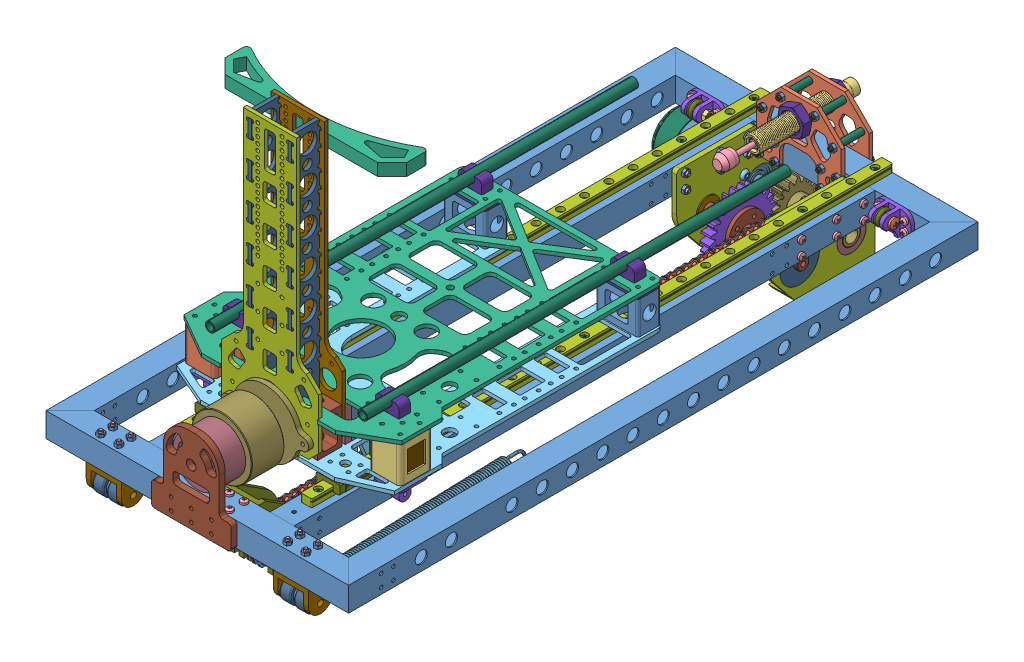
SolidWorks assembly 寒冰射手-wlⅡ-2AT-sc, configuration 默认. Lengths in mm.
Overall size (250 317.6 547).
340 component instances, 60 part files, 291 mates.
Components (placement in the parent):
- 发射架-wlⅡ-2AT-sc-1: 发射架-wlⅡ-2AT-sc [默认<按加工>] at (-51.2492 42.8186 0) size (250 20 520)
- 缓冲器固定板-wlⅡ-2AT-sc-1: 缓冲器固定板-wlⅡ-2AT-sc [默认] at (-86.2492 32.8186 -263) x (1 0 0) z (0 -1 0) size (70 3 58)
- 缓冲器固定板-wlⅡ-2AT-sc-3: 缓冲器固定板-wlⅡ-2AT-sc [默认] at (-86.2492 32.8186 -240) x (1 0 0) z (0 -1 0) size (70 3 58)
- 阻尼器-wlⅡ-2AT-sc-1: 阻尼器-wlⅡ-2AT-sc [默认] at (5.2053 79.9344 -231.7218) x (0.997955 0.063917 0) z (0.063917 -0.997955 0) size (16.63 112.5 16.63)
  - 阻尼器缸体-wlⅡ-2AT-sc-1: 阻尼器缸体-wlⅡ-2AT-sc [默认] at (-56.5702 -50.2782 0) size (16.17 84.55 14.32)
  - 阻尼器杆-wlⅡ-2AT-sc-1: 阻尼器杆-wlⅡ-2AT-sc [默认] at (-56.5702 14.7218 0) x (0.905287 0 0.424801) z (-0.424801 0 0.905287) size (12.5 47.5 12.5)
  - GB／T70．1-2000内六角圆柱头螺钉M4×20-wlⅡ-2AT-sc-1: GB／T70．1-2000内六角圆柱头螺钉M4×20-wlⅡ-2AT-sc [默认] at (-56.5702 -49.2782 0) x (0 1 0) z (0.698141 0 0.715961) size (24 7 7)
  - circlips for holes--type a gb-1: circlips for holes--type a gb [GB_CONNECTING_PIECE_RING_RRH 10] at (-56.5702 31.0218 0) x (1 0 0) z (0 1 0) size (10.8 10.39 0.8)
- 发射导轨-wlⅡ-2AT-sc-1: 发射导轨-wlⅡ-2AT-sc [默认] at (-1.2492 56.482 -260) size (9 6.5 480)
- 发射导轨-wlⅡ-2AT-sc-2: 发射导轨-wlⅡ-2AT-sc [默认] at (-101.2492 56.482 -260) size (9 6.5 480)
- 拉线座子-wlⅡ-2AT-sc-1: 拉线座子-wlⅡ-2AT-sc [默认] at (26.0008 25.8186 -231.5) x (-1 0 0) z (0 0 -1) size (30.5 20 17)
- 拉线座子-wlⅡ-2AT-sc-2: 拉线座子-wlⅡ-2AT-sc [默认] at (-128.4992 25.8186 -231.5) x (-1 0 0) z (0 0 -1) size (30.5 20 17)
- 拉簧座子-wlⅡ-2AT-sc-1: 拉簧座子-wlⅡ-2AT-sc [默认] at (26.0008 32.8186 250) x (0 0 -1) z (0 -1 0) size (20 29 22)
- 拉簧座子-wlⅡ-2AT-sc-2: 拉簧座子-wlⅡ-2AT-sc [默认] at (-128.4992 32.8186 250) x (0 0 -1) z (0 -1 0) size (20 29 22)
- 弹簧限位件-wlⅡ-2AT-sc-1: 弹簧限位件-wlⅡ-2AT-sc [Default] at (-129.9992 18.3186 250) x (0 0.381849 -0.924225) z (0 0.924225 0.381849) size (18 9 18)
- 弹簧限位件-wlⅡ-2AT-sc-2: 弹簧限位件-wlⅡ-2AT-sc [Default] at (-117.9992 18.3186 250) x (0 0.381849 -0.924225) z (0 0.924225 0.381849) size (18 9 18)
- 弹簧限位件-wlⅡ-2AT-sc-3: 弹簧限位件-wlⅡ-2AT-sc [Default] at (36.5008 18.3186 250) x (0 0.381849 -0.924225) z (0 0.924225 0.381849) size (18 9 18)
- 弹簧限位件-wlⅡ-2AT-sc-4: 弹簧限位件-wlⅡ-2AT-sc [Default] at (24.5008 18.3186 250) x (0 0.381849 -0.924225) z (0 0.924225 0.381849) size (18 9 18)
- 电磁吸盘固定板-wlⅡ-2AT-sc-1: 电磁吸盘固定板-wlⅡ-2AT-sc [默认] at (-51.2492 67.8186 265) x (1 0 0) z (0 1 0) size (66 5 70)
- 电磁铁开关80kg-wlⅡ-2AT-sc-1: 电磁铁开关80kg-wlⅡ-2AT-sc [默认] at (-51.2492 78.8186 213) x (-0.910179 -0.414215 0) z (-0.414215 0.910179 0) size (50 27 50)
- 行程调节块-wlⅡ-2AT-sc-1: 行程调节块-wlⅡ-2AT-sc [默认] at (-51.2492 78.8186 240) x (1 0 0) z (0 -1 0) size (40 20 40)
- 拉射拉簧-wlⅡ-2AT-sc-1: 拉射拉簧-wlⅡ-2AT-sc [默认] at (-128.4992 23.8376 81.5904) x (1 0 0) z (0 -0.999461 -0.032825) size (15 191.85 17.32)
- 拉射拉簧-wlⅡ-2AT-sc-2: 拉射拉簧-wlⅡ-2AT-sc [默认] at (26.0008 23.8376 81.5904) x (1 0 0) z (0 -0.999461 -0.032825) size (15 191.85 17.32)
- 20尼龙柱-wlⅡ-2AT-sc-1: 20尼龙柱-wlⅡ-2AT-sc [默认] at (-65.1781 84.8186 -240) x (1 0 0) z (0 1 0) size (5 20 5)
- 20尼龙柱-wlⅡ-2AT-sc-2: 20尼龙柱-wlⅡ-2AT-sc [默认] at (-22.2492 69.7475 -240) x (1 0 0) z (0 1 0) size (5 20 5)
- 20尼龙柱-wlⅡ-2AT-sc-3: 20尼龙柱-wlⅡ-2AT-sc [默认] at (-80.2492 69.7475 -240) x (1 0 0) z (0 1 0) size (5 20 5)
- 20尼龙柱-wlⅡ-2AT-sc-4: 20尼龙柱-wlⅡ-2AT-sc [默认] at (-37.3203 84.8186 -240) x (1 0 0) z (0 1 0) size (5 20 5)
- 现有线轮轴承-wlⅡ-2AT-sc-1: 现有线轮轴承-wlⅡ-2AT-sc [默认] at (-128.4992 46.0686 -231) x (1 0 0) z (0 0.011922 0.999929) size (6 13 13)
- 现有线轮轴承-wlⅡ-2AT-sc-2: 现有线轮轴承-wlⅡ-2AT-sc [默认] at (26.0008 46.0686 -231) x (1 0 0) z (0 -0.105623 0.994406) size (6 13 13)
- GB／T6172．1-2000六角薄螺母A级和B级(M14)-wlⅡ-2AT-sc-1: GB／T6172．1-2000六角薄螺母A级和B级(M14)-wlⅡ-2AT-sc [默认] at (-51.2492 76.3186 -270) x (0.985088 -0.17205 0) z (0 0 1) size (20.46 23.35 7)
- GB／T6172．1-2000六角薄螺母A级和B级(M14)-wlⅡ-2AT-sc-2: GB／T6172．1-2000六角薄螺母A级和B级(M14)-wlⅡ-2AT-sc [默认] at (-51.2492 76.3186 -237) x (0.985088 -0.17205 0) z (0 0 1) size (20.46 23.35 7)
- GB／T818-2000十字槽盘头螺钉M3×30-wlⅡ-2AT-sc-1: GB／T818-2000十字槽盘头螺钉M3×30-wlⅡ-2AT-sc [默认] at (-65.1781 84.8186 -265.4) x (0 0 1) z (-0.574659 -0.818393 0) size (32.39 5.6 5.6)
- GB／T818-2000十字槽盘头螺钉M3×30-wlⅡ-2AT-sc-2: GB／T818-2000十字槽盘头螺钉M3×30-wlⅡ-2AT-sc [默认] at (-80.2492 69.7475 -265.4) x (0 0 1) z (-0.574659 -0.818393 0) size (32.39 5.6 5.6)
- GB／T818-2000十字槽盘头螺钉M3×30-wlⅡ-2AT-sc-3: GB／T818-2000十字槽盘头螺钉M3×30-wlⅡ-2AT-sc [默认] at (-37.3203 84.8186 -265.4) x (0 0 1) z (-0.144538 -0.989499 0) size (32.39 5.6 5.6)
- GB／T818-2000十字槽盘头螺钉M3×30-wlⅡ-2AT-sc-4: GB／T818-2000十字槽盘头螺钉M3×30-wlⅡ-2AT-sc [默认] at (-22.2492 69.7475 -265.4) x (0 0 1) z (-0.574659 -0.818393 0) size (32.39 5.6 5.6)
- GB／T818-2000十字槽盘头螺钉M3×30-wlⅡ-2AT-sc-6: GB／T818-2000十字槽盘头螺钉M3×30-wlⅡ-2AT-sc [默认] at (-19.2492 35.8186 -265.4) x (0 0 1) z (-0.574659 -0.818393 0) size (32.39 5.6 5.6)
- GB／T818-2000十字槽盘头螺钉M3×30-wlⅡ-2AT-sc-7: GB／T818-2000十字槽盘头螺钉M3×30-wlⅡ-2AT-sc [默认] at (-32.2492 35.8186 -265.4) x (0 0 1) z (-0.574659 -0.818393 0) size (32.39 5.6 5.6)
- GB／T818-2000十字槽盘头螺钉M3×30-wlⅡ-2AT-sc-8: GB／T818-2000十字槽盘头螺钉M3×30-wlⅡ-2AT-sc [默认] at (-70.2492 35.8186 -265.4) x (0 0 1) z (-0.574659 -0.818393 0) size (32.39 5.6 5.6)
- GB／T818-2000十字槽盘头螺钉M3×30-wlⅡ-2AT-sc-9: GB／T818-2000十字槽盘头螺钉M3×30-wlⅡ-2AT-sc [默认] at (-70.2492 49.8186 -265.4) x (0 0 1) z (-0.187811 -0.982205 0) size (32.39 5.6 5.6)
- GB／T818-2000十字槽盘头螺钉M3×30-wlⅡ-2AT-sc-10: GB／T818-2000十字槽盘头螺钉M3×30-wlⅡ-2AT-sc [默认] at (-32.2492 49.8186 -265.4) x (0 0 1) z (-0.574659 -0.818393 0) size (32.39 5.6 5.6)
- GB／T818-2000十字槽盘头螺钉M3×30-wlⅡ-2AT-sc-11: GB／T818-2000十字槽盘头螺钉M3×30-wlⅡ-2AT-sc [默认] at (-83.2492 35.8186 -265.4) x (0 0 1) z (-0.574659 -0.818393 0) size (32.39 5.6 5.6)
- GB／T818-2000十字槽盘头螺钉M3×30-wlⅡ-2AT-sc-12: GB／T818-2000十字槽盘头螺钉M3×30-wlⅡ-2AT-sc [默认] at (-83.2492 49.8186 -265.4) x (0 0 1) z (-0.574659 -0.818393 0) size (32.39 5.6 5.6)
- GB／T818-2000十字槽盘头螺钉M3×30-wlⅡ-2AT-sc-13: GB／T818-2000十字槽盘头螺钉M3×30-wlⅡ-2AT-sc [默认] at (-19.2492 49.8186 -265.4) x (0 0 1) z (-0.574659 -0.818393 0) size (32.39 5.6 5.6)
- GB／T6170-20001型六角螺母A级和B级M3-wlⅡ-2AT-sc-1: GB／T6170-20001型六角螺母A级和B级M3-wlⅡ-2AT-sc [默认] at (-19.2492 35.8186 -237) size (5.25 6.01 2.4)
- GB／T6170-20001型六角螺母A级和B级M3-wlⅡ-2AT-sc-2: GB／T6170-20001型六角螺母A级和B级M3-wlⅡ-2AT-sc [默认] at (-32.2492 35.8186 -237) size (5.25 6.01 2.4)
- GB／T6170-20001型六角螺母A级和B级M3-wlⅡ-2AT-sc-4: GB／T6170-20001型六角螺母A级和B级M3-wlⅡ-2AT-sc [默认] at (-70.2492 35.8186 -237) size (5.25 6.01 2.4)
- GB／T6170-20001型六角螺母A级和B级M3-wlⅡ-2AT-sc-5: GB／T6170-20001型六角螺母A级和B级M3-wlⅡ-2AT-sc [默认] at (-83.2492 35.8186 -237) size (5.25 6.01 2.4)
- GB／T6170-20001型六角螺母A级和B级M3-wlⅡ-2AT-sc-6: GB／T6170-20001型六角螺母A级和B级M3-wlⅡ-2AT-sc [默认] at (-83.2492 49.8186 -237) size (5.25 6.01 2.4)
- GB／T6170-20001型六角螺母A级和B级M3-wlⅡ-2AT-sc-7: GB／T6170-20001型六角螺母A级和B级M3-wlⅡ-2AT-sc [默认] at (-70.2492 49.8186 -237) size (5.25 6.01 2.4)
- GB／T6170-20001型六角螺母A级和B级M3-wlⅡ-2AT-sc-8: GB／T6170-20001型六角螺母A级和B级M3-wlⅡ-2AT-sc [默认] at (-80.2492 69.7475 -237) size (5.25 6.01 2.4)
- GB／T6170-20001型六角螺母A级和B级M3-wlⅡ-2AT-sc-9: GB／T6170-20001型六角螺母A级和B级M3-wlⅡ-2AT-sc [默认] at (-65.1781 84.8186 -237) size (5.25 6.01 2.4)
- GB／T6170-20001型六角螺母A级和B级M3-wlⅡ-2AT-sc-11: GB／T6170-20001型六角螺母A级和B级M3-wlⅡ-2AT-sc [默认] at (-32.2492 49.8186 -237) size (5.25 6.01 2.4)
- GB／T6170-20001型六角螺母A级和B级M3-wlⅡ-2AT-sc-12: GB／T6170-20001型六角螺母A级和B级M3-wlⅡ-2AT-sc [默认] at (-19.2492 49.8186 -237) size (5.25 6.01 2.4)
- GB／T6170-20001型六角螺母A级和B级M3-wlⅡ-2AT-sc-13: GB／T6170-20001型六角螺母A级和B级M3-wlⅡ-2AT-sc [默认] at (-37.3203 84.8186 -237) size (5.25 6.01 2.4)
- GB／T6170-20001型六角螺母A级和B级M3-wlⅡ-2AT-sc-14: GB／T6170-20001型六角螺母A级和B级M3-wlⅡ-2AT-sc [默认] at (-22.2492 69.7475 -237) size (5.25 6.01 2.4)
- GB／T818-2000十字槽盘头螺钉M4×16-wlⅡ-2AT-sc-1: GB／T818-2000十字槽盘头螺钉M4×16-wlⅡ-2AT-sc [默认] at (-137.8492 46.0686 -231) x (1 0 0) z (0 -0.572973 0.819575) size (19.08 8 8)
- GB／T818-2000十字槽盘头螺钉M4×16-wlⅡ-2AT-sc-2: GB／T818-2000十字槽盘头螺钉M4×16-wlⅡ-2AT-sc [默认] at (35.3508 46.0686 -231) x (-1 0 0) z (0 -0.995405 -0.095753) size (19.08 8 8)
- GB／T6170-20001型六角螺母A级和B级M4-wlⅡ-2AT-sc-1: GB／T6170-20001型六角螺母A级和B级M4-wlⅡ-2AT-sc [默认] at (-119.0492 46.0686 -231) x (0 0 1) z (-1 0 0) size (6.73 7.66 3.2)
- GB／T6170-20001型六角螺母A级和B级M4-wlⅡ-2AT-sc-2: GB／T6170-20001型六角螺母A级和B级M4-wlⅡ-2AT-sc [默认] at (19.7508 46.0686 -231) x (0 0 1) z (-1 0 0) size (6.73 7.66 3.2)
- GB／T818-2000十字槽盘头螺钉M3×28-wlⅡ-2AT-sc-1: GB／T818-2000十字槽盘头螺钉M3×28-wlⅡ-2AT-sc [默认] at (11.1508 48.8186 -230) x (-1 0 0) z (0 -0.776163 -0.630532) size (30.39 5.6 5.6)
- GB／T818-2000十字槽盘头螺钉M3×28-wlⅡ-2AT-sc-2: GB／T818-2000十字槽盘头螺钉M3×28-wlⅡ-2AT-sc [默认] at (11.1508 36.8186 -230) x (-1 0 0) z (0 -0.776163 -0.630532) size (30.39 5.6 5.6)
- GB／T818-2000十字槽盘头螺钉M3×28-wlⅡ-2AT-sc-3: GB／T818-2000十字槽盘头螺钉M3×28-wlⅡ-2AT-sc [默认] at (11.1508 36.8186 -207.5) x (-1 0 0) z (0 -0.776163 -0.630532) size (30.39 5.6 5.6)
- GB／T818-2000十字槽盘头螺钉M3×28-wlⅡ-2AT-sc-4: GB／T818-2000十字槽盘头螺钉M3×28-wlⅡ-2AT-sc [默认] at (11.1508 48.8186 -207.5) x (-1 0 0) z (0 -0.776163 -0.630532) size (30.39 5.6 5.6)
- GB／T818-2000十字槽盘头螺钉M3×28-wlⅡ-2AT-sc-5: GB／T818-2000十字槽盘头螺钉M3×28-wlⅡ-2AT-sc [默认] at (11.1508 48.8186 -178.5) x (-1 0 0) z (0 -0.776163 -0.630532) size (30.39 5.6 5.6)
- GB／T818-2000十字槽盘头螺钉M3×28-wlⅡ-2AT-sc-6: GB／T818-2000十字槽盘头螺钉M3×28-wlⅡ-2AT-sc [默认] at (11.1508 36.8186 -178.5) x (-1 0 0) z (0 -0.776163 -0.630532) size (30.39 5.6 5.6)
- GB／T818-2000十字槽盘头螺钉M3×28-wlⅡ-2AT-sc-7: GB／T818-2000十字槽盘头螺钉M3×28-wlⅡ-2AT-sc [默认] at (-113.6492 36.8186 -178.5) x (1 0 0) z (0 -0.032657 0.999467) size (30.39 5.6 5.6)
- GB／T818-2000十字槽盘头螺钉M3×28-wlⅡ-2AT-sc-8: GB／T818-2000十字槽盘头螺钉M3×28-wlⅡ-2AT-sc [默认] at (-113.6492 48.8186 -178.5) x (1 0 0) z (0 -0.032657 0.999467) size (30.39 5.6 5.6)
- GB／T818-2000十字槽盘头螺钉M3×28-wlⅡ-2AT-sc-9: GB／T818-2000十字槽盘头螺钉M3×28-wlⅡ-2AT-sc [默认] at (-113.6492 36.8186 -207.5) x (1 0 0) z (0 -0.032657 0.999467) size (30.39 5.6 5.6)
- GB／T818-2000十字槽盘头螺钉M3×28-wlⅡ-2AT-sc-10: GB／T818-2000十字槽盘头螺钉M3×28-wlⅡ-2AT-sc [默认] at (-113.6492 48.8186 -207.5) x (1 0 0) z (0 -0.032657 0.999467) size (30.39 5.6 5.6)
- GB／T818-2000十字槽盘头螺钉M3×28-wlⅡ-2AT-sc-11: GB／T818-2000十字槽盘头螺钉M3×28-wlⅡ-2AT-sc [默认] at (-113.6492 48.8186 -230) x (1 0 0) z (0 0.032028 0.999487) size (30.39 5.6 5.6)
- GB／T818-2000十字槽盘头螺钉M3×28-wlⅡ-2AT-sc-12: GB／T818-2000十字槽盘头螺钉M3×28-wlⅡ-2AT-sc [默认] at (-113.6492 36.8186 -230) x (1 0 0) z (0 -0.032657 0.999467) size (30.39 5.6 5.6)
- GB／T6170-20001型六角螺母A级和B级M3-wlⅡ-2AT-sc-15: GB／T6170-20001型六角螺母A级和B级M3-wlⅡ-2AT-sc [默认] at (-17.6492 48.8186 -230) x (0 -0.145643 -0.989337) z (1 0 0) size (5.25 6.01 2.4)
- GB／T6170-20001型六角螺母A级和B级M3-wlⅡ-2AT-sc-16: GB／T6170-20001型六角螺母A级和B级M3-wlⅡ-2AT-sc [默认] at (-17.6492 36.8186 -230) x (0 -0.263585 -0.964636) z (1 0 0) size (5.25 6.01 2.4)
- GB／T6170-20001型六角螺母A级和B级M3-wlⅡ-2AT-sc-17: GB／T6170-20001型六角螺母A级和B级M3-wlⅡ-2AT-sc [默认] at (-17.6492 48.8186 -207.5) x (0 -0.006116 -0.999981) z (1 0 0) size (5.25 6.01 2.4)
- GB／T6170-20001型六角螺母A级和B级M3-wlⅡ-2AT-sc-18: GB／T6170-20001型六角螺母A级和B级M3-wlⅡ-2AT-sc [默认] at (-17.6492 36.8186 -207.5) x (0 -0.595602 -0.80328) z (1 0 0) size (5.25 6.01 2.4)
- GB／T6170-20001型六角螺母A级和B级M3-wlⅡ-2AT-sc-19: GB／T6170-20001型六角螺母A级和B级M3-wlⅡ-2AT-sc [默认] at (-17.6492 48.8186 -178.5) x (0 -0.668571 -0.743649) z (1 0 0) size (5.25 6.01 2.4)
- GB／T6170-20001型六角螺母A级和B级M3-wlⅡ-2AT-sc-20: GB／T6170-20001型六角螺母A级和B级M3-wlⅡ-2AT-sc [默认] at (-17.6492 36.8186 -178.5) x (0 -0.388181 -0.921583) z (1 0 0) size (5.25 6.01 2.4)
- GB／T6170-20001型六角螺母A级和B级M3-wlⅡ-2AT-sc-21: GB／T6170-20001型六角螺母A级和B级M3-wlⅡ-2AT-sc [默认] at (-87.2492 48.8186 -178.5) x (0 0.010585 -0.999944) z (1 0 0) size (5.25 6.01 2.4)
- GB／T6170-20001型六角螺母A级和B级M3-wlⅡ-2AT-sc-23: GB／T6170-20001型六角螺母A级和B级M3-wlⅡ-2AT-sc [默认] at (-87.2492 36.8186 -178.5) x (0 -0.892194 0.451652) z (1 0 0) size (5.25 6.01 2.4)
- GB／T6170-20001型六角螺母A级和B级M3-wlⅡ-2AT-sc-24: GB／T6170-20001型六角螺母A级和B级M3-wlⅡ-2AT-sc [默认] at (-87.2492 36.8186 -230) x (0 0.351908 0.936034) z (1 0 0) size (5.25 6.01 2.4)
- GB／T6170-20001型六角螺母A级和B级M3-wlⅡ-2AT-sc-26: GB／T6170-20001型六角螺母A级和B级M3-wlⅡ-2AT-sc [默认] at (-87.2492 48.8186 -207.5) x (0 0.644572 0.764544) z (1 0 0) size (5.25 6.01 2.4)
- GB／T6170-20001型六角螺母A级和B级M3-wlⅡ-2AT-sc-27: GB／T6170-20001型六角螺母A级和B级M3-wlⅡ-2AT-sc [默认] at (-87.2492 48.8186 -230) x (0 0.518332 0.855179) z (1 0 0) size (5.25 6.01 2.4)
- GB／T6170-20001型六角螺母A级和B级M3-wlⅡ-2AT-sc-28: GB／T6170-20001型六角螺母A级和B级M3-wlⅡ-2AT-sc [默认] at (-87.2492 36.8186 -207.5) x (0 0.371561 0.928408) z (1 0 0) size (5.25 6.01 2.4)
- GB／T70．2-2000内六角平圆头螺钉M4×12-wlⅡ-2AT-sc-1: GB／T70．2-2000内六角平圆头螺钉M4×12-wlⅡ-2AT-sc [默认] at (-99.2492 -1.9942 -253.1998) x (-1 0 0) z (0 -0.978952 0.204093) size (14.38 7.6 7.6)
- GB／T70．2-2000内六角平圆头螺钉M4×12-wlⅡ-2AT-sc-2: GB／T70．2-2000内六角平圆头螺钉M4×12-wlⅡ-2AT-sc [默认] at (-99.2492 22.7491 -252.682) x (-1 0 0) z (0 -0.978952 0.204093) size (14.38 7.6 7.6)
- GB／T70．2-2000内六角平圆头螺钉M4×12-wlⅡ-2AT-sc-3: GB／T70．2-2000内六角平圆头螺钉M4×12-wlⅡ-2AT-sc [默认] at (-99.2492 22.2313 -227.9387) x (-1 0 0) z (0 -0.978952 0.204093) size (14.38 7.6 7.6)
- GB／T70．2-2000内六角平圆头螺钉M4×12-wlⅡ-2AT-sc-4: GB／T70．2-2000内六角平圆头螺钉M4×12-wlⅡ-2AT-sc [默认] at (-99.2492 -2.512 -228.4565) x (-1 0 0) z (0 -0.978952 0.204093) size (14.38 7.6 7.6)
- GB／T818-2000十字槽盘头螺钉M3×28-wlⅡ-2AT-sc-13: GB／T818-2000十字槽盘头螺钉M3×28-wlⅡ-2AT-sc [默认] at (-117.7492 46.8186 -234.6) x (0 0 -1) z (0.940908 0.338663 0) size (30.39 5.6 5.6)
- GB／T818-2000十字槽盘头螺钉M3×28-wlⅡ-2AT-sc-14: GB／T818-2000十字槽盘头螺钉M3×28-wlⅡ-2AT-sc [默认] at (-139.2492 38.8186 -234.6) x (0 0 -1) z (0.940908 0.338663 0) size (30.39 5.6 5.6)
- GB／T818-2000十字槽盘头螺钉M3×28-wlⅡ-2AT-sc-15: GB／T818-2000十字槽盘头螺钉M3×28-wlⅡ-2AT-sc [默认] at (-117.7492 38.8186 -234.6) x (0 0 -1) z (0.940908 0.338663 0) size (30.39 5.6 5.6)
- GB／T818-2000十字槽盘头螺钉M3×28-wlⅡ-2AT-sc-16: GB／T818-2000十字槽盘头螺钉M3×28-wlⅡ-2AT-sc [默认] at (-139.2492 46.8186 -234.6) x (0 0 -1) z (0.940908 0.338663 0) size (30.39 5.6 5.6)
- GB／T818-2000十字槽盘头螺钉M3×28-wlⅡ-2AT-sc-17: GB／T818-2000十字槽盘头螺钉M3×28-wlⅡ-2AT-sc [默认] at (15.2508 46.8186 -234.6) x (0 0 -1) z (0.739289 -0.673388 0) size (30.39 5.6 5.6)
- GB／T818-2000十字槽盘头螺钉M3×28-wlⅡ-2AT-sc-18: GB／T818-2000十字槽盘头螺钉M3×28-wlⅡ-2AT-sc [默认] at (36.7508 46.8186 -234.6) x (0 0 -1) z (0.940908 0.338663 0) size (30.39 5.6 5.6)
- GB／T818-2000十字槽盘头螺钉M3×28-wlⅡ-2AT-sc-19: GB／T818-2000十字槽盘头螺钉M3×28-wlⅡ-2AT-sc [默认] at (15.2508 38.8186 -234.6) x (0 0 -1) z (0.940908 0.338663 0) size (30.39 5.6 5.6)
- GB／T818-2000十字槽盘头螺钉M3×28-wlⅡ-2AT-sc-20: GB／T818-2000十字槽盘头螺钉M3×28-wlⅡ-2AT-sc [默认] at (36.7508 38.8186 -234.6) x (0 0 -1) z (0.940908 0.338663 0) size (30.39 5.6 5.6)
- GB／T6170-20001型六角螺母A级和B级M3-wlⅡ-2AT-sc-29: GB／T6170-20001型六角螺母A级和B级M3-wlⅡ-2AT-sc [默认] at (36.7508 38.8186 -262.4) x (-0.867986 0.49659 0) z (0 0 1) size (5.25 6.01 2.4)
- GB／T6170-20001型六角螺母A级和B级M3-wlⅡ-2AT-sc-30: GB／T6170-20001型六角螺母A级和B级M3-wlⅡ-2AT-sc [默认] at (36.7508 46.8186 -262.4) x (-0.867986 0.49659 0) z (0 0 1) size (5.25 6.01 2.4)
- GB／T6170-20001型六角螺母A级和B级M3-wlⅡ-2AT-sc-31: GB／T6170-20001型六角螺母A级和B级M3-wlⅡ-2AT-sc [默认] at (15.2508 38.8186 -262.4) x (-0.867986 0.49659 0) z (0 0 1) size (5.25 6.01 2.4)
- GB／T6170-20001型六角螺母A级和B级M3-wlⅡ-2AT-sc-32: GB／T6170-20001型六角螺母A级和B级M3-wlⅡ-2AT-sc [默认] at (15.2508 46.8186 -262.4) x (-0.867986 0.49659 0) z (0 0 1) size (5.25 6.01 2.4)
- GB／T6170-20001型六角螺母A级和B级M3-wlⅡ-2AT-sc-33: GB／T6170-20001型六角螺母A级和B级M3-wlⅡ-2AT-sc [默认] at (-117.7492 38.8186 -262.4) x (-0.867986 0.49659 0) z (0 0 1) size (5.25 6.01 2.4)
- GB／T6170-20001型六角螺母A级和B级M3-wlⅡ-2AT-sc-34: GB／T6170-20001型六角螺母A级和B级M3-wlⅡ-2AT-sc [默认] at (-139.2492 38.8186 -262.4) x (-0.867986 0.49659 0) z (0 0 1) size (5.25 6.01 2.4)
- GB／T6170-20001型六角螺母A级和B级M3-wlⅡ-2AT-sc-35: GB／T6170-20001型六角螺母A级和B级M3-wlⅡ-2AT-sc [默认] at (-117.7492 46.8186 -262.4) x (-0.867986 0.49659 0) z (0 0 1) size (5.25 6.01 2.4)
- GB／T6170-20001型六角螺母A级和B级M3-wlⅡ-2AT-sc-36: GB／T6170-20001型六角螺母A级和B级M3-wlⅡ-2AT-sc [默认] at (-139.2492 46.8186 -262.4) x (-0.867986 0.49659 0) z (0 0 1) size (5.25 6.01 2.4)
- GB／T818-2000十字槽盘头螺钉M3×25-wlⅡ-2AT-sc-1: GB／T818-2000十字槽盘头螺钉M3×25-wlⅡ-2AT-sc [默认] at (-1.2492 58.2186 -190) x (0 -1 0) z (-0.435623 0 0.900129) size (27.39 5.6 5.6)
- GB／T818-2000十字槽盘头螺钉M3×25-wlⅡ-2AT-sc-2: GB／T818-2000十字槽盘头螺钉M3×25-wlⅡ-2AT-sc [默认] at (-101.2492 58.2186 -190) x (0 -1 0) z (-0.990452 0 0.137855) size (27.39 5.6 5.6)
- GB／T818-2000十字槽盘头螺钉M3×25-wlⅡ-2AT-sc-3: GB／T818-2000十字槽盘头螺钉M3×25-wlⅡ-2AT-sc [默认] at (-101.2492 58.2186 -250) x (0 -1 0) z (0.985919 0 0.167221) size (27.39 5.6 5.6)
- GB／T818-2000十字槽盘头螺钉M3×25-wlⅡ-2AT-sc-4: GB／T818-2000十字槽盘头螺钉M3×25-wlⅡ-2AT-sc [默认] at (-1.2492 58.2186 -250) x (0 -1 0) z (-0.400002 0 0.916514) size (27.39 5.6 5.6)
- GB／T818-2000十字槽盘头螺钉M3×25-wlⅡ-2AT-sc-5: GB／T818-2000十字槽盘头螺钉M3×25-wlⅡ-2AT-sc [默认] at (-1.2492 58.2186 -10) x (0 -1 0) z (0.775986 0 -0.630751) size (27.39 5.6 5.6)
- GB／T818-2000十字槽盘头螺钉M3×25-wlⅡ-2AT-sc-6: GB／T818-2000十字槽盘头螺钉M3×25-wlⅡ-2AT-sc [默认] at (-101.2492 58.2186 -10) x (0 -1 0) z (0.985919 0 0.167221) size (27.39 5.6 5.6)
- GB／T818-2000十字槽盘头螺钉M3×25-wlⅡ-2AT-sc-7: GB／T818-2000十字槽盘头螺钉M3×25-wlⅡ-2AT-sc [默认] at (-1.2492 58.2186 210) x (0 -1 0) z (0.985919 0 0.167221) size (27.39 5.6 5.6)
- GB／T818-2000十字槽盘头螺钉M3×25-wlⅡ-2AT-sc-8: GB／T818-2000十字槽盘头螺钉M3×25-wlⅡ-2AT-sc [默认] at (-101.2492 58.2186 210) x (0 -1 0) z (0.985919 0 0.167221) size (27.39 5.6 5.6)
- GB／T6170-20001型六角螺母A级和B级M3-wlⅡ-2AT-sc-37: GB／T6170-20001型六角螺母A级和B级M3-wlⅡ-2AT-sc [默认] at (-101.2492 30.4186 -190) x (0 0 -1) z (0 1 0) size (5.25 6.01 2.4)
- GB／T6170-20001型六角螺母A级和B级M3-wlⅡ-2AT-sc-38: GB／T6170-20001型六角螺母A级和B级M3-wlⅡ-2AT-sc [默认] at (-101.2492 30.4186 -250) x (0 0 -1) z (0 1 0) size (5.25 6.01 2.4)
- GB／T6170-20001型六角螺母A级和B级M3-wlⅡ-2AT-sc-39: GB／T6170-20001型六角螺母A级和B级M3-wlⅡ-2AT-sc [默认] at (-1.2492 30.4186 -250) x (0 0 -1) z (0 1 0) size (5.25 6.01 2.4)
- GB／T6170-20001型六角螺母A级和B级M3-wlⅡ-2AT-sc-40: GB／T6170-20001型六角螺母A级和B级M3-wlⅡ-2AT-sc [默认] at (-1.2492 30.4186 -190) x (0 0 -1) z (0 1 0) size (5.25 6.01 2.4)
- GB／T6170-20001型六角螺母A级和B级M3-wlⅡ-2AT-sc-41: GB／T6170-20001型六角螺母A级和B级M3-wlⅡ-2AT-sc [默认] at (-1.2492 30.4186 -10) x (0 0 -1) z (0 1 0) size (5.25 6.01 2.4)
- GB／T6170-20001型六角螺母A级和B级M3-wlⅡ-2AT-sc-42: GB／T6170-20001型六角螺母A级和B级M3-wlⅡ-2AT-sc [默认] at (-101.2492 30.4186 -10) x (0 0 -1) z (0 1 0) size (5.25 6.01 2.4)
- GB／T6170-20001型六角螺母A级和B级M3-wlⅡ-2AT-sc-43: GB／T6170-20001型六角螺母A级和B级M3-wlⅡ-2AT-sc [默认] at (-101.2492 30.4186 210) x (0 0 -1) z (0 1 0) size (5.25 6.01 2.4)
- GB／T6170-20001型六角螺母A级和B级M3-wlⅡ-2AT-sc-44: GB／T6170-20001型六角螺母A级和B级M3-wlⅡ-2AT-sc [默认] at (-1.2492 30.4186 210) x (0 0 -1) z (0 1 0) size (5.25 6.01 2.4)
- GB／T818-2000十字槽盘头螺钉M3×28-wlⅡ-2AT-sc-21: GB／T818-2000十字槽盘头螺钉M3×28-wlⅡ-2AT-sc [默认] at (-135.9992 26.4186 245) x (0 1 0) z (0.032657 0 0.999467) size (30.39 5.6 5.6)
- GB／T818-2000十字槽盘头螺钉M3×28-wlⅡ-2AT-sc-22: GB／T818-2000十字槽盘头螺钉M3×28-wlⅡ-2AT-sc [默认] at (-135.9992 26.4186 255) x (0 1 0) z (0.032657 0 0.999467) size (30.39 5.6 5.6)
- GB／T818-2000十字槽盘头螺钉M3×28-wlⅡ-2AT-sc-23: GB／T818-2000十字槽盘头螺钉M3×28-wlⅡ-2AT-sc [默认] at (-120.9992 26.4186 255) x (0 1 0) z (0.032657 0 0.999467) size (30.39 5.6 5.6)
- GB／T818-2000十字槽盘头螺钉M3×28-wlⅡ-2AT-sc-24: GB／T818-2000十字槽盘头螺钉M3×28-wlⅡ-2AT-sc [默认] at (-120.9992 26.4186 245) x (0 1 0) z (-0.73452 0 0.678587) size (30.39 5.6 5.6)
- GB／T818-2000十字槽盘头螺钉M3×28-wlⅡ-2AT-sc-25: GB／T818-2000十字槽盘头螺钉M3×28-wlⅡ-2AT-sc [默认] at (18.5008 26.4186 255) x (0 1 0) z (0.032657 0 0.999467) size (30.39 5.6 5.6)
- GB／T818-2000十字槽盘头螺钉M3×28-wlⅡ-2AT-sc-26: GB／T818-2000十字槽盘头螺钉M3×28-wlⅡ-2AT-sc [默认] at (33.5008 26.4186 245) x (0 1 0) z (0.032657 0 0.999467) size (30.39 5.6 5.6)
- GB／T818-2000十字槽盘头螺钉M3×28-wlⅡ-2AT-sc-27: GB／T818-2000十字槽盘头螺钉M3×28-wlⅡ-2AT-sc [默认] at (33.5008 26.4186 255) x (0 1 0) z (0.032657 0 0.999467) size (30.39 5.6 5.6)
- GB／T818-2000十字槽盘头螺钉M3×28-wlⅡ-2AT-sc-28: GB／T818-2000十字槽盘头螺钉M3×28-wlⅡ-2AT-sc [默认] at (18.5008 26.4186 245) x (0 1 0) z (0.032657 0 0.999467) size (30.39 5.6 5.6)
- GB／T818-2000十字槽盘头螺钉M3×28-wlⅡ-2AT-sc-29: GB／T818-2000十字槽盘头螺钉M3×28-wlⅡ-2AT-sc [默认] at (-28.6492 55.2186 244) x (0 -1 0) z (-0.573992 0 0.818861) size (30.39 5.6 5.6)
- GB／T818-2000十字槽盘头螺钉M3×28-wlⅡ-2AT-sc-30: GB／T818-2000十字槽盘头螺钉M3×28-wlⅡ-2AT-sc [默认] at (-40.6492 55.2186 244) x (0 -1 0) z (0.999087 0 0.042726) size (30.39 5.6 5.6)
- GB／T818-2000十字槽盘头螺钉M3×28-wlⅡ-2AT-sc-31: GB／T818-2000十字槽盘头螺钉M3×28-wlⅡ-2AT-sc [默认] at (-40.6492 55.2186 256) x (0 -1 0) z (-0.573992 0 0.818861) size (30.39 5.6 5.6)
- GB／T818-2000十字槽盘头螺钉M3×28-wlⅡ-2AT-sc-32: GB／T818-2000十字槽盘头螺钉M3×28-wlⅡ-2AT-sc [默认] at (-28.6492 55.2186 256) x (0 -1 0) z (-0.573992 0 0.818861) size (30.39 5.6 5.6)
- GB／T6170-20001型六角螺母A级和B级M3-wlⅡ-2AT-sc-46: GB／T6170-20001型六角螺母A级和B级M3-wlⅡ-2AT-sc [默认] at (-28.6492 26.4186 256) x (0 0 -1) z (0 1 0) size (5.25 6.01 2.4)
- GB／T6170-20001型六角螺母A级和B级M3-wlⅡ-2AT-sc-47: GB／T6170-20001型六角螺母A级和B级M3-wlⅡ-2AT-sc [默认] at (-28.6492 26.4186 244) x (0 0 -1) z (0 1 0) size (5.25 6.01 2.4)
- GB／T6170-20001型六角螺母A级和B级M3-wlⅡ-2AT-sc-48: GB／T6170-20001型六角螺母A级和B级M3-wlⅡ-2AT-sc [默认] at (-40.6492 26.4186 244) x (0 0 -1) z (0 1 0) size (5.25 6.01 2.4)
- GB／T6170-20001型六角螺母A级和B级M3-wlⅡ-2AT-sc-49: GB／T6170-20001型六角螺母A级和B级M3-wlⅡ-2AT-sc [默认] at (-40.6492 26.4186 256) x (0 0 -1) z (0 1 0) size (5.25 6.01 2.4)
- GB／T6170-20001型六角螺母A级和B级M3-wlⅡ-2AT-sc-50: GB／T6170-20001型六角螺母A级和B级M3-wlⅡ-2AT-sc [默认] at (18.5008 52.8186 245) x (-0.54717 0 0.837021) z (0 1 0) size (5.25 6.01 2.4)
- GB／T6170-20001型六角螺母A级和B级M3-wlⅡ-2AT-sc-51: GB／T6170-20001型六角螺母A级和B级M3-wlⅡ-2AT-sc [默认] at (33.5008 52.8186 245) x (-0.729205 0 0.684295) z (0 1 0) size (5.25 6.01 2.4)
- GB／T6170-20001型六角螺母A级和B级M3-wlⅡ-2AT-sc-52: GB／T6170-20001型六角螺母A级和B级M3-wlⅡ-2AT-sc [默认] at (18.5008 52.8186 255) x (-0.011354 0 -0.999936) z (0 1 0) size (5.25 6.01 2.4)
- GB／T6170-20001型六角螺母A级和B级M3-wlⅡ-2AT-sc-53: GB／T6170-20001型六角螺母A级和B级M3-wlⅡ-2AT-sc [默认] at (33.5008 52.8186 255) x (0 0 -1) z (0 1 0) size (5.25 6.01 2.4)
- GB／T6170-20001型六角螺母A级和B级M3-wlⅡ-2AT-sc-54: GB／T6170-20001型六角螺母A级和B级M3-wlⅡ-2AT-sc [默认] at (-135.9992 52.8186 255) x (-0.127372 0 0.991855) z (0 1 0) size (5.25 6.01 2.4)
- GB／T6170-20001型六角螺母A级和B级M3-wlⅡ-2AT-sc-55: GB／T6170-20001型六角螺母A级和B级M3-wlⅡ-2AT-sc [默认] at (-135.9992 52.8186 245) x (-0.568546 0 0.822651) z (0 1 0) size (5.25 6.01 2.4)
- GB／T6170-20001型六角螺母A级和B级M3-wlⅡ-2AT-sc-56: GB／T6170-20001型六角螺母A级和B级M3-wlⅡ-2AT-sc [默认] at (-120.9992 52.8186 255) x (-0.93749 0 0.348011) z (0 1 0) size (5.25 6.01 2.4)
- GB／T6170-20001型六角螺母A级和B级M3-wlⅡ-2AT-sc-57: GB／T6170-20001型六角螺母A级和B级M3-wlⅡ-2AT-sc [默认] at (-120.9992 52.8186 245) x (-0.426065 0 0.904693) z (0 1 0) size (5.25 6.01 2.4)
- 主动链轮模块T-sc-1: 主动链轮模块T-sc [默认] at (29.405 16.0951 -256.9298) x (0 0.264538 -0.964375) z (1 0 0) size (109.92 88.41 154.8)
  - 电机固定架T-sc-1: 电机固定架T-sc [默认] at (-30.0887 -0.3286 -120.6542) x (0.964375 -0.264538 0) z (0 0 1) size (88 66 80)
  - 圆柱齿轮26×2   -wlⅡ-2AT-sc-1: 圆柱齿轮26×2   -wlⅡ-2AT-sc [默认] at (-58.0116 12.5156 -95.1542) x (0.787383 0.616464 0) z (0 0 1) size (56 55.75 8)
  - F10X19X5-wlⅡ-2AT-sc-1: F10X19X5-wlⅡ-2AT-sc [默认] at (-58.0116 12.5156 -115.6542) x (-0.25312 0.967435 0) z (0 0 -1) size (21 21 5)
  - F10X30X9T-wlⅡ-2AT-sc-1: F10X30X9T-wlⅡ-2AT-sc [默认] at (-58.0116 12.5156 -49.6542) x (-0.735572 0.677447 0) z (0 0 1) size (32.5 32.5 9)
  - 链轮轴04CT-sc-2: 链轮轴04CT-sc [默认] at (-58.0116 12.5156 -62.6542) x (-0.616464 0.787383 0) z (0 0 -1) size (36.98 36.84 86)
  - 圆柱齿轮轴17×2T-sc-1: 圆柱齿轮轴17×2T-sc [默认] at (-17.4381 -1.7249 -86.1542) x (-0.612977 0.7901 0) z (0 0 -1) size (38.05 37.79 73)
  - F15X24X5T-wlⅡ-2AT-sc-1: F15X24X5T-wlⅡ-2AT-sc [默认] at (-17.4381 -1.7249 -40.7542) x (0.874702 0.484661 0) z (0 0 -1) size (26 26 5)
  - 3508 电机。。4465TYZQL116K12-wlⅡ-2AT-sc-1: 3508 电机。。4465TYZQL116K12-wlⅡ-2AT-sc [默认] at (-23.6884 7.244 -48.9042) x (-0.512932 0.858429 0) z (0 0 -1) size (53.91 53.91 98.8) (flexible)
    - 3508减速。。4465TYZQL116K12-wlⅡ-2AT-sc-2: 3508减速。。4465TYZQL116K12-wlⅡ-2AT-sc [默认] at (-10.9051 0.765 71.75) size (42 42 75.5)
    - 3508电机屁股。。4465TYZQL116K12-wlⅡ-2AT-sc-2: 3508电机屁股。。4465TYZQL116K12-wlⅡ-2AT-sc [默认] at (-10.9051 0.765 120.85) x (-0.938585 -0.345048 0) z (0 0 1) size (42 42 22.7)
- 从动链轮模块T-sc-1: 从动链轮模块T-sc [默认] at (51.2553 -13.1679 212.8857) x (1 0 0) z (0 1 0) size (36 63.73 58.75)
  - 链轮座T-sc-1: 链轮座T-sc [默认] at (-121.9045 -25.1143 77.9865) size (28 60 56)
  - F10X19X5-wlⅡ-2AT-sc-1: F10X19X5-wlⅡ-2AT-sc [默认] at (-95.9045 -2.1143 25.9869) x (0 0.43527 0.9003) z (-1 0 0) size (21 21 5)
  - F10X19X5-wlⅡ-2AT-sc-2: F10X19X5-wlⅡ-2AT-sc [默认] at (-75.9045 -2.1143 25.9869) x (0 -0.973892 0.227011) z (1 0 0) size (21 21 5)
  - 从动链轮轴T-wlⅡ-2AT-sc-1: 从动链轮轴T-wlⅡ-2AT-sc [默认] at (-84.5045 -2.1143 25.9869) x (0 -0.013321 0.999911) z (-1 0 0) size (18.6 18.6 36)
  - 从动链轮T-sc-1: 从动链轮T-sc [默认] at (-84.5045 -2.1143 25.9869) x (0 0.999911 0.013321) z (-1 0 0) size (36.98 36.84 3)
- 外链板T-sc-1: 外链板T-sc [默认] at (-37.9392 28.1337 -205.0066) x (0 0.255572 0.96679) z (1 0 0) size (12.35 6 8.2)
- 内链板T-sc-1: 内链板T-sc [默认] at (-33.1592 29.7566 -198.8675) x (0 0.0072 0.999974) z (1 0 0) size (12.35 6 4.78)
- 外链板T-sc-2: 外链板T-sc [默认] at (-37.9392 29.8023 -192.5177) x (0 0.000728 1) z (1 0 0) size (12.35 6 8.2)
- 外链板T-sc-3: 外链板T-sc [默认] at (-37.9392 29.8115 -179.8177) x (0 0.000728 1) z (1 0 0) size (12.35 6 8.2)
- 外链板T-sc-4: 外链板T-sc [默认] at (-37.9392 29.8208 -167.1177) x (0 0.000728 1) z (1 0 0) size (12.35 6 8.2)
- 外链板T-sc-5: 外链板T-sc [默认] at (-37.9392 29.83 -154.4177) x (0 0.000728 1) z (1 0 0) size (12.35 6 8.2)
- 外链板T-sc-6: 外链板T-sc [默认] at (-37.9392 29.8393 -141.7177) x (0 0.000728 1) z (1 0 0) size (12.35 6 8.2)
- 外链板T-sc-7: 外链板T-sc [默认] at (-37.9392 29.8485 -129.0177) x (0 0.000728 1) z (1 0 0) size (12.35 6 8.2)
- 外链板T-sc-8: 外链板T-sc [默认] at (-37.9392 29.8578 -116.3177) x (0 0.000728 1) z (1 0 0) size (12.35 6 8.2)
- 外链板T-sc-9: 外链板T-sc [默认] at (-37.9392 29.867 -103.6177) x (0 0.000728 1) z (1 0 0) size (12.35 6 8.2)
- 外链板T-sc-10: 外链板T-sc [默认] at (-37.9392 29.8763 -90.9178) x (0 0.000728 1) z (1 0 0) size (12.35 6 8.2)
- 外链板T-sc-11: 外链板T-sc [默认] at (-37.9392 29.8855 -78.2178) x (0 0.000728 1) z (1 0 0) size (12.35 6 8.2)
- 外链板T-sc-12: 外链板T-sc [默认] at (-37.9392 29.8947 -65.5178) x (0 0.000728 1) z (1 0 0) size (12.35 6 8.2)
- 外链板T-sc-13: 外链板T-sc [默认] at (-37.9392 29.904 -52.8178) x (0 0.000728 1) z (1 0 0) size (12.35 6 8.2)
- 外链板T-sc-14: 外链板T-sc [默认] at (-37.9392 29.9132 -40.1178) x (0 0.000728 1) z (1 0 0) size (12.35 6 8.2)
- 外链板T-sc-15: 外链板T-sc [默认] at (-37.9392 29.9225 -27.4178) x (0 0.000728 1) z (1 0 0) size (12.35 6 8.2)
- 外链板T-sc-16: 外链板T-sc [默认] at (-37.9392 29.9317 -14.7178) x (0 0.000728 1) z (1 0 0) size (12.35 6 8.2)
- 外链板T-sc-17: 外链板T-sc [默认] at (-37.9392 29.941 -2.0178) x (0 0.000728 1) z (1 0 0) size (12.35 6 8.2)
- 外链板T-sc-18: 外链板T-sc [默认] at (-37.9392 29.9502 10.6822) x (0 0.000728 1) z (1 0 0) size (12.35 6 8.2)
- 外链板T-sc-19: 外链板T-sc [默认] at (-37.9392 29.9595 23.3821) x (0 0.000728 1) z (1 0 0) size (12.35 6 8.2)
- 外链板T-sc-20: 外链板T-sc [默认] at (-37.9392 29.9687 36.0821) x (0 0.000728 1) z (1 0 0) size (12.35 6 8.2)
- 外链板T-sc-21: 外链板T-sc [默认] at (-37.9392 29.978 48.7821) x (0 0.000728 1) z (1 0 0) size (12.35 6 8.2)
- 外链板T-sc-22: 外链板T-sc [默认] at (-37.9392 29.9872 61.4821) x (0 0.000728 1) z (1 0 0) size (12.35 6 8.2)
- 外链板T-sc-23: 外链板T-sc [默认] at (-37.9392 29.9964 74.1821) x (0 0.000728 1) z (1 0 0) size (12.35 6 8.2)
- 外链板T-sc-24: 外链板T-sc [默认] at (-37.9392 30.0057 86.8821) x (0 0.000728 1) z (1 0 0) size (12.35 6 8.2)
- 外链板T-sc-25: 外链板T-sc [默认] at (-37.9392 30.0149 99.5821) x (0 0.000728 1) z (1 0 0) size (12.35 6 8.2)
- 外链板T-sc-26: 外链板T-sc [默认] at (-37.9392 30.0242 112.2821) x (0 0.000728 1) z (1 0 0) size (12.35 6 8.2)
- 外链板T-sc-27: 外链板T-sc [默认] at (-37.9392 30.0334 124.9821) x (0 0.000728 1) z (1 0 0) size (12.35 6 8.2)
- 外链板T-sc-28: 外链板T-sc [默认] at (-37.9392 30.0427 137.6821) x (0 0.000728 1) z (1 0 0) size (12.35 6 8.2)
- 外链板T-sc-29: 外链板T-sc [默认] at (-37.9392 30.0519 150.382) x (0 0.000728 1) z (1 0 0) size (12.35 6 8.2)
- 外链板T-sc-30: 外链板T-sc [默认] at (-37.9392 30.0612 163.082) x (0 0.000728 1) z (1 0 0) size (12.35 6 8.2)
- 外链板T-sc-31: 外链板T-sc [默认] at (-37.9392 30.0704 175.782) x (0 0.000728 1) z (1 0 0) size (12.35 6 8.2)
- 外链板T-sc-32: 外链板T-sc [默认] at (-37.9392 30.0797 188.482) x (0 0.000728 1) z (1 0 0) size (12.35 6 8.2)
- 外链板T-sc-33: 外链板T-sc [默认] at (-37.9392 30.0889 201.182) x (0 0.000728 1) z (1 0 0) size (12.35 6 8.2)
- 外链板T-sc-34: 外链板T-sc [默认] at (-37.9392 30.0981 213.882) x (0 -0.125121 0.992142) z (1 0 0) size (12.35 6 8.2)
- 外链板T-sc-35: 外链板T-sc [默认] at (-37.9392 26.3187 225.7868) x (0 -0.757151 0.653239) z (1 0 0) size (12.35 6 8.2)
- 外链板T-sc-36: 外链板T-sc [默认] at (-37.9392 15.5292 232.0661) x (0 -0.999627 -0.027294) z (1 0 0) size (12.35 6 8.2)
- 外链板T-sc-37: 外链板T-sc [默认] at (-37.9392 3.3251 229.4383) x (0 -0.720377 -0.693583) z (1 0 0) size (12.35 6 8.2)
- 外链板T-sc-38: 外链板T-sc [默认] at (-37.9392 -3.9239 219.2748) x (0 -0.084351 -0.996436) z (1 0 0) size (12.35 6 8.2)
- 外链板T-sc-39: 外链板T-sc [默认] at (-37.9392 -4.4549 206.5975) x (0 0.000726 -1) z (1 0 0) size (12.35 6 8.2)
- 外链板T-sc-40: 外链板T-sc [默认] at (-37.9392 -4.4457 193.8975) x (0 0.000726 -1) z (1 0 0) size (12.35 6 8.2)
- 外链板T-sc-41: 外链板T-sc [默认] at (-37.9392 -4.4365 181.1975) x (0 0.000726 -1) z (1 0 0) size (12.35 6 8.2)
- 外链板T-sc-42: 外链板T-sc [默认] at (-37.9392 -4.4273 168.4975) x (0 0.000726 -1) z (1 0 0) size (12.35 6 8.2)
- 外链板T-sc-43: 外链板T-sc [默认] at (-37.9392 -4.4181 155.7975) x (0 0.000726 -1) z (1 0 0) size (12.35 6 8.2)
- 外链板T-sc-44: 外链板T-sc [默认] at (-37.9392 -4.4088 143.0975) x (0 0.000726 -1) z (1 0 0) size (12.35 6 8.2)
- 外链板T-sc-45: 外链板T-sc [默认] at (-37.9392 -4.3996 130.3975) x (0 0.000726 -1) z (1 0 0) size (12.35 6 8.2)
- 外链板T-sc-46: 外链板T-sc [默认] at (-37.9392 -4.3904 117.6975) x (0 0.000726 -1) z (1 0 0) size (12.35 6 8.2)
- 外链板T-sc-47: 外链板T-sc [默认] at (-37.9392 -4.3812 104.9975) x (0 0.000726 -1) z (1 0 0) size (12.35 6 8.2)
- 外链板T-sc-48: 外链板T-sc [默认] at (-37.9392 -4.372 92.2976) x (0 0.000726 -1) z (1 0 0) size (12.35 6 8.2)
- 外链板T-sc-49: 外链板T-sc [默认] at (-37.9392 -4.3627 79.5976) x (0 0.000726 -1) z (1 0 0) size (12.35 6 8.2)
- 外链板T-sc-50: 外链板T-sc [默认] at (-37.9392 -4.3535 66.8976) x (0 0.000726 -1) z (1 0 0) size (12.35 6 8.2)
- 外链板T-sc-51: 外链板T-sc [默认] at (-37.9392 -4.3443 54.1976) x (0 0.000726 -1) z (1 0 0) size (12.35 6 8.2)
- 外链板T-sc-52: 外链板T-sc [默认] at (-37.9392 -4.3351 41.4976) x (0 0.000726 -1) z (1 0 0) size (12.35 6 8.2)
- 外链板T-sc-53: 外链板T-sc [默认] at (-37.9392 -4.3259 28.7976) x (0 0.000726 -1) z (1 0 0) size (12.35 6 8.2)
- 外链板T-sc-54: 外链板T-sc [默认] at (-37.9392 -4.3166 16.0976) x (0 0.000726 -1) z (1 0 0) size (12.35 6 8.2)
- 外链板T-sc-55: 外链板T-sc [默认] at (-37.9392 -4.3074 3.3976) x (0 0.000726 -1) z (1 0 0) size (12.35 6 8.2)
- 外链板T-sc-56: 外链板T-sc [默认] at (-37.9392 -4.2982 -9.3024) x (0 0.000726 -1) z (1 0 0) size (12.35 6 8.2)
- 外链板T-sc-57: 外链板T-sc [默认] at (-37.9392 -4.289 -22.0023) x (0 0.000726 -1) z (1 0 0) size (12.35 6 8.2)
- 外链板T-sc-58: 外链板T-sc [默认] at (-37.9392 -4.2798 -34.7023) x (0 0.000726 -1) z (1 0 0) size (12.35 6 8.2)
- 外链板T-sc-59: 外链板T-sc [默认] at (-37.9392 -4.2705 -47.4023) x (0 0.000726 -1) z (1 0 0) size (12.35 6 8.2)
- 外链板T-sc-60: 外链板T-sc [默认] at (-37.9392 -4.2613 -60.1023) x (0 0.000726 -1) z (1 0 0) size (12.35 6 8.2)
- 外链板T-sc-61: 外链板T-sc [默认] at (-37.9392 -4.2521 -72.8023) x (0 0.000726 -1) z (1 0 0) size (12.35 6 8.2)
- 外链板T-sc-62: 外链板T-sc [默认] at (-37.9392 -4.2429 -85.5023) x (0 0.000726 -1) z (1 0 0) size (12.35 6 8.2)
- 外链板T-sc-63: 外链板T-sc [默认] at (-37.9392 -4.2336 -98.2023) x (0 0.000726 -1) z (1 0 0) size (12.35 6 8.2)
- 外链板T-sc-64: 外链板T-sc [默认] at (-37.9392 -4.2244 -110.9023) x (0 0.000726 -1) z (1 0 0) size (12.35 6 8.2)
- 外链板T-sc-65: 外链板T-sc [默认] at (-37.9392 -4.2152 -123.6023) x (0 0.000726 -1) z (1 0 0) size (12.35 6 8.2)
- 外链板T-sc-66: 外链板T-sc [默认] at (-37.9392 -4.206 -136.3023) x (0 0.000726 -1) z (1 0 0) size (12.35 6 8.2)
- 外链板T-sc-67: 外链板T-sc [默认] at (-37.9392 -4.1968 -149.0022) x (0 0.000726 -1) z (1 0 0) size (12.35 6 8.2)
- 外链板T-sc-68: 外链板T-sc [默认] at (-37.9392 -4.1875 -161.7022) x (0 0.000726 -1) z (1 0 0) size (12.35 6 8.2)
- 外链板T-sc-69: 外链板T-sc [默认] at (-37.9392 -4.1783 -174.4022) x (0 0.000726 -1) z (1 0 0) size (12.35 6 8.2)
- 外链板T-sc-70: 外链板T-sc [默认] at (-37.9392 -4.1691 -187.1022) x (0 0.000726 -1) z (1 0 0) size (12.35 6 8.2)
- 外链板T-sc-71: 外链板T-sc [默认] at (-37.9392 -4.0277 -199.8007) x (0 0.308553 -0.951207) z (1 0 0) size (12.35 6 8.2)
- 外链板T-sc-72: 外链板T-sc [默认] at (-37.9392 1.9729 -210.7389) x (0 0.875292 -0.483595) z (1 0 0) size (12.35 6 8.2)
- 外链板T-sc-73: 外链板T-sc [默认] at (-37.9392 13.8286 -214.6239) x (0 0.969501 0.245087) z (1 0 0) size (12.35 6 8.2)
- 内链板T-sc-2: 内链板T-sc [默认] at (-33.1592 29.8069 -186.1677) x (0 0.000728 1) z (1 0 0) size (12.35 6 4.78)
- 内链板T-sc-3: 内链板T-sc [默认] at (-33.1592 29.8162 -173.4677) x (0 0.000728 1) z (1 0 0) size (12.35 6 4.78)
- 内链板T-sc-4: 内链板T-sc [默认] at (-33.1592 29.8254 -160.7677) x (0 0.000728 1) z (1 0 0) size (12.35 6 4.78)
- 内链板T-sc-5: 内链板T-sc [默认] at (-33.1592 29.8347 -148.0677) x (0 0.000728 1) z (1 0 0) size (12.35 6 4.78)
- 内链板T-sc-6: 内链板T-sc [默认] at (-33.1592 29.8439 -135.3677) x (0 0.000728 1) z (1 0 0) size (12.35 6 4.78)
- 内链板T-sc-7: 内链板T-sc [默认] at (-33.1592 29.8531 -122.6677) x (0 0.000728 1) z (1 0 0) size (12.35 6 4.78)
- 内链板T-sc-8: 内链板T-sc [默认] at (-33.1592 29.8624 -109.9677) x (0 0.000728 1) z (1 0 0) size (12.35 6 4.78)
- 内链板T-sc-9: 内链板T-sc [默认] at (-33.1592 29.8716 -97.2678) x (0 0.000728 1) z (1 0 0) size (12.35 6 4.78)
- 内链板T-sc-10: 内链板T-sc [默认] at (-33.1592 29.8809 -84.5678) x (0 0.000728 1) z (1 0 0) size (12.35 6 4.78)
- 内链板T-sc-11: 内链板T-sc [默认] at (-33.1592 29.8901 -71.8678) x (0 0.000728 1) z (1 0 0) size (12.35 6 4.78)
- 内链板T-sc-12: 内链板T-sc [默认] at (-33.1592 29.8994 -59.1678) x (0 0.000728 1) z (1 0 0) size (12.35 6 4.78)
- 内链板T-sc-13: 内链板T-sc [默认] at (-33.1592 29.9086 -46.4678) x (0 0.000728 1) z (1 0 0) size (12.35 6 4.78)
- 内链板T-sc-14: 内链板T-sc [默认] at (-33.1592 29.9179 -33.7678) x (0 0.000728 1) z (1 0 0) size (12.35 6 4.78)
- 内链板T-sc-15: 内链板T-sc [默认] at (-33.1592 29.9271 -21.0678) x (0 0.000728 1) z (1 0 0) size (12.35 6 4.78)
- 内链板T-sc-16: 内链板T-sc [默认] at (-33.1592 29.9364 -8.3678) x (0 0.000728 1) z (1 0 0) size (12.35 6 4.78)
- 内链板T-sc-17: 内链板T-sc [默认] at (-33.1592 29.9456 4.3322) x (0 0.000728 1) z (1 0 0) size (12.35 6 4.78)
- 内链板T-sc-18: 内链板T-sc [默认] at (-33.1592 29.9548 17.0322) x (0 0.000728 1) z (1 0 0) size (12.35 6 4.78)
- 内链板T-sc-19: 内链板T-sc [默认] at (-33.1592 29.9641 29.7321) x (0 0.000728 1) z (1 0 0) size (12.35 6 4.78)
- 内链板T-sc-20: 内链板T-sc [默认] at (-33.1592 29.9733 42.4321) x (0 0.000728 1) z (1 0 0) size (12.35 6 4.78)
- 内链板T-sc-21: 内链板T-sc [默认] at (-33.1592 29.9826 55.1321) x (0 0.000728 1) z (1 0 0) size (12.35 6 4.78)
- 内链板T-sc-22: 内链板T-sc [默认] at (-33.1592 29.9918 67.8321) x (0 0.000728 1) z (1 0 0) size (12.35 6 4.78)
- 内链板T-sc-23: 内链板T-sc [默认] at (-33.1592 30.0011 80.5321) x (0 0.000728 1) z (1 0 0) size (12.35 6 4.78)
- 内链板T-sc-24: 内链板T-sc [默认] at (-33.1592 30.0103 93.2321) x (0 0.000728 1) z (1 0 0) size (12.35 6 4.78)
- 内链板T-sc-25: 内链板T-sc [默认] at (-33.1592 30.0196 105.9321) x (0 0.000728 1) z (1 0 0) size (12.35 6 4.78)
- 内链板T-sc-26: 内链板T-sc [默认] at (-33.1592 30.0288 118.6321) x (0 0.000728 1) z (1 0 0) size (12.35 6 4.78)
